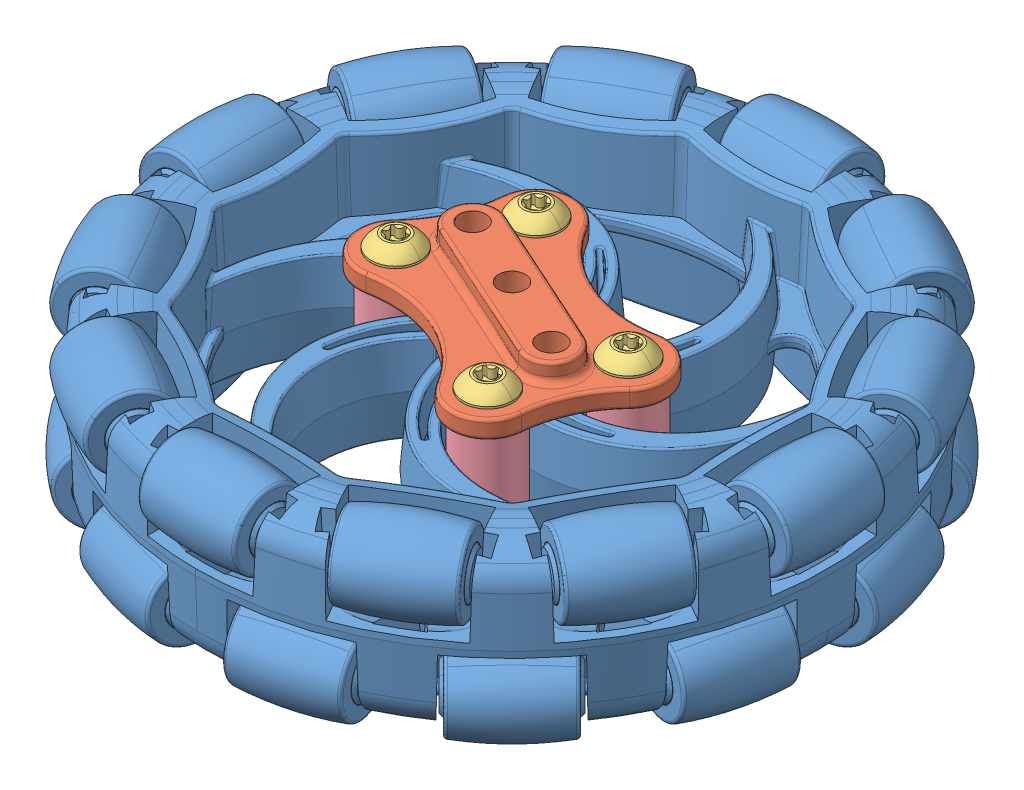
SolidWorks assembly ChassisWheel, configuration Default. Lengths in mm.
Overall size (114.44 40.55 114.44).
10 component instances, 4 part files, 19 mates.
Components (placement in the parent):
- 4_ Omni-Directional Wheel (276-2185) -1: 4_ Omni-Directional Wheel (276-2185)  [Default] at (37.9935 59.5978 90.4079) size (114.44 40.55 114.44)
- wheel_gear_mount-1: wheel_gear_mount [Default] at (37.9935 69.1228 90.4079) x (0.911659 0 0.410949) z (-0.410949 0 0.911659) size (41.65 6 29.12)
- #8-32 x 1.000_ Star Drive Screw (276-4996)-1: #8-32 x 1.000_ Star Drive Screw (276-4996) [Default] at (55.0259 72.1228 88.6971) size (7.92 27.61 7.92)
- #8-32 x 1.000_ Star Drive Screw (276-4996)-2: #8-32 x 1.000_ Star Drive Screw (276-4996) [Default] at (27.9958 72.1228 76.5128) size (7.92 27.61 7.92)
- #8-32 x 1.000_ Star Drive Screw (276-4996)-3: #8-32 x 1.000_ Star Drive Screw (276-4996) [Default] at (20.9612 72.1228 92.1186) size (7.92 27.61 7.92)
- #8-32 x 1.000_ Star Drive Screw (276-4996)-4: #8-32 x 1.000_ Star Drive Screw (276-4996) [Default] at (47.9912 72.1228 104.303) size (7.92 27.61 7.92)
- wheel_lock_spacer-1: wheel_lock_spacer [Default] at (47.9912 69.1228 104.303) x (1 0 0) z (0 -1 0) size (9.53 9.53 19.05)
- wheel_lock_spacer-2: wheel_lock_spacer [Default] at (55.0259 69.1228 88.6971) x (1 0 0) z (0 -1 0) size (9.53 9.53 19.05)
- wheel_lock_spacer-3: wheel_lock_spacer [Default] at (27.9958 69.1228 76.5128) x (1 0 0) z (0 -1 0) size (9.53 9.53 19.05)
- wheel_lock_spacer-4: wheel_lock_spacer [Default] at (20.9612 50.0728 92.1186) x (1 0 0) z (0 1 0) size (9.53 9.53 19.05)
Mates (geometry in assembly coordinates):
- Concentric1: concentric aligned: cone of 4_ Omni-Directional Wheel (276-2185) -1 through (37.9935 68.8281 90.4079) axis (0 -1 0); cylinder of wheel_gear_mount-1 through (37.9935 72.1228 90.4079) axis (0 -1 0) radius 2.15
- Coincident1: coincident anti-aligned: plane of 4_ Omni-Directional Wheel (276-2185) -1 through (37.9935 69.1228 90.4079) normal (0 1 0); plane of wheel_gear_mount-1 through (20.9612 69.1228 92.1186) normal (0 -1 0)
- Concentric2: concentric anti-aligned: cylinder of wheel_gear_mount-1 through (55.0259 72.1228 88.6971) axis (0 -1 0) radius 2.15; cylinder of #8-32 x 1.000_ Star Drive Screw (276-4996)-1 through (55.0259 46.7228 88.6971) axis (0 1 0) radius 2.0828
- Coincident2: coincident anti-aligned: plane of wheel_gear_mount-1 through (20.9612 72.1228 92.1186) normal (0 1 0); plane of #8-32 x 1.000_ Star Drive Screw (276-4996)-1 through (55.0259 72.1228 88.6971) normal (0 -1 0)
- Concentric3: concentric anti-aligned: cylinder of wheel_gear_mount-1 through (27.9958 72.1228 76.5128) axis (0 -1 0) radius 2.15; cylinder of #8-32 x 1.000_ Star Drive Screw (276-4996)-2 through (27.9958 46.7228 76.5128) axis (0 1 0) radius 2.0828
- Concentric4: concentric anti-aligned: cylinder of wheel_gear_mount-1 through (20.9612 72.1228 92.1186) axis (0 -1 0) radius 2.15; cylinder of #8-32 x 1.000_ Star Drive Screw (276-4996)-3 through (20.9612 46.7228 92.1186) axis (0 1 0) radius 2.0828
- Concentric5: concentric anti-aligned: cylinder of wheel_gear_mount-1 through (47.9912 72.1228 104.303) axis (0 -1 0) radius 2.15; cylinder of #8-32 x 1.000_ Star Drive Screw (276-4996)-4 through (47.9912 46.7228 104.303) axis (0 1 0) radius 2.0828
- Coincident3: coincident anti-aligned: plane of wheel_gear_mount-1 through (20.9612 72.1228 92.1186) normal (0 1 0); plane of #8-32 x 1.000_ Star Drive Screw (276-4996)-4 through (47.9912 72.1228 104.303) normal (0 -1 0)
- Coincident4: coincident anti-aligned: plane of wheel_gear_mount-1 through (20.9612 72.1228 92.1186) normal (0 1 0); plane of #8-32 x 1.000_ Star Drive Screw (276-4996)-3 through (20.9612 72.1228 92.1186) normal (0 -1 0)
- Coincident5: coincident anti-aligned: plane of wheel_gear_mount-1 through (20.9612 72.1228 92.1186) normal (0 1 0); plane of #8-32 x 1.000_ Star Drive Screw (276-4996)-2 through (27.9958 72.1228 76.5128) normal (0 -1 0)
- Coincident6: coincident anti-aligned: plane of wheel_gear_mount-1 through (20.9612 69.1228 92.1186) normal (0 -1 0); plane of wheel_lock_spacer-1 through (47.9912 69.1228 104.303) normal (0 1 0)
- Concentric6: concentric aligned: cylinder of #8-32 x 1.000_ Star Drive Screw (276-4996)-4 through (47.9912 46.7228 104.303) axis (0 1 0) radius 2.0828; cylinder of wheel_lock_spacer-1 through (47.9912 50.0728 104.303) axis (0 1 0) radius 2.25
- Tangent1: tangent: curve of 4_ Omni-Directional Wheel (276-2185) -1; cylinder of wheel_lock_spacer-1 through (47.9912 50.0728 104.303) axis (0 1 0) radius 4.7625
- Coincident7: coincident anti-aligned: plane of wheel_gear_mount-1 through (20.9612 69.1228 92.1186) normal (0 -1 0); plane of wheel_lock_spacer-2 through (55.0259 69.1228 88.6971) normal (0 1 0)
- Concentric7: concentric aligned: cylinder of #8-32 x 1.000_ Star Drive Screw (276-4996)-1 through (55.0259 46.7228 88.6971) axis (0 1 0) radius 2.0828; cylinder of wheel_lock_spacer-2 through (55.0259 50.0728 88.6971) axis (0 1 0) radius 2.25
- Coincident8: coincident anti-aligned: plane of wheel_gear_mount-1 through (20.9612 69.1228 92.1186) normal (0 -1 0); plane of wheel_lock_spacer-3 through (27.9958 69.1228 76.5128) normal (0 1 0)
- Concentric8: concentric aligned: cylinder of #8-32 x 1.000_ Star Drive Screw (276-4996)-2 through (27.9958 46.7228 76.5128) axis (0 1 0) radius 2.0828; cylinder of wheel_lock_spacer-3 through (27.9958 50.0728 76.5128) axis (0 1 0) radius 2.25
- Coincident9: coincident anti-aligned: plane of wheel_gear_mount-1 through (20.9612 69.1228 92.1186) normal (0 -1 0); plane of wheel_lock_spacer-4 through (20.9612 69.1228 92.1186) normal (0 1 0)
- Concentric9: concentric anti-aligned: cylinder of #8-32 x 1.000_ Star Drive Screw (276-4996)-3 through (20.9612 46.7228 92.1186) axis (0 1 0) radius 2.0828; cylinder of wheel_lock_spacer-4 through (20.9612 69.1228 92.1186) axis (0 -1 0) radius 2.25
